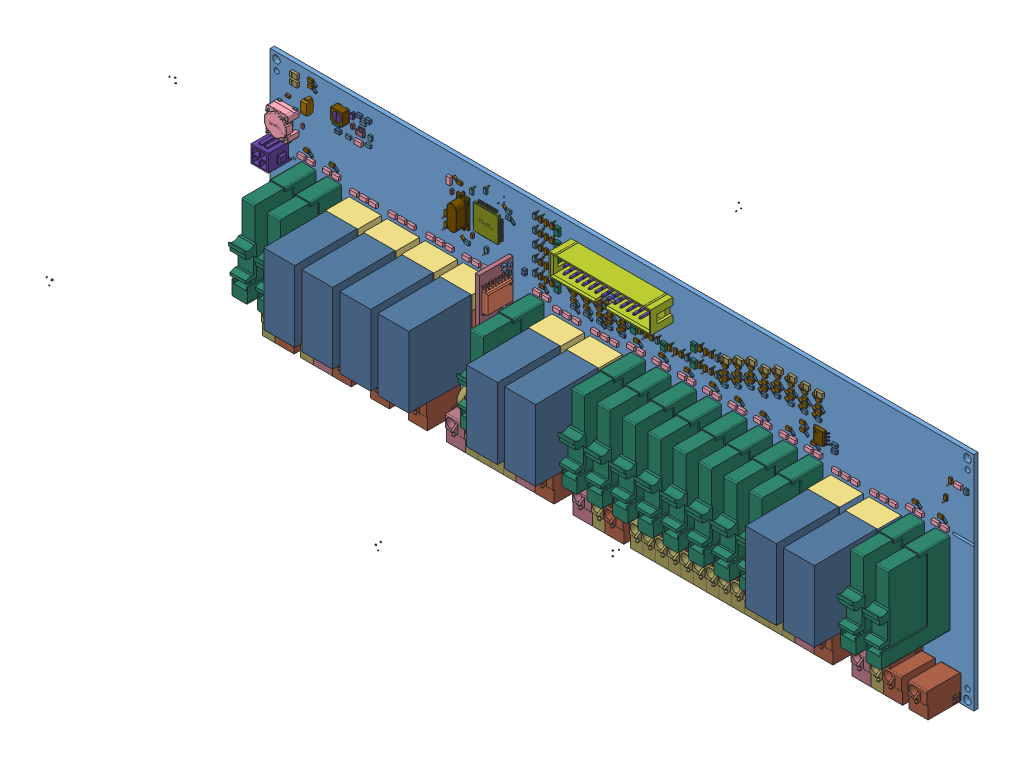
SolidWorks assembly _SC941C, configuration Default. Lengths in mm. (continued)
Components (placement in the parent): (continued)
- R40-1: R40 [Default] at origin size (1.97 3.3 0.78)
  - SW3dPS-0805_SMD_Resistor-1: SW3dPS-0805_SMD_Resistor [Default] at (147.4471 56.8959 0) x (0 -1 0) z (-1 0 0) size (2 0.78 1.25)
  - 905262864-1: 905262864 [Default] at (148.1217 58.6819 0) size (1.35 1.03 0.76)
    - Extruded_11-1: Extruded_11 [Default] at origin size (1.35 1.03 0.76)
  - 905261368-1: 905261368 [Default] at (148.0423 58.4438 0) size (1.51 1.51 0.76)
    - Extruded_12-1: Extruded_12 [Default] at origin size (1.51 1.51 0.76)
  - 905260688-1: 905260688 [Default] at (148.082 58.5629 0) size (1.43 1.11 0.76)
    - Extruded_13-1: Extruded_13 [Default] at origin size (1.43 1.11 0.76)
- R35-1: R35 [Default] at origin size (3.3 1.97 0.78)
  - SW3dPS-0805_SMD_Resistor-1: SW3dPS-0805_SMD_Resistor [Default] at (130.8101 54.2291 0) x (1 0 0) z (0 -1 0) size (2 0.78 1.25)
  - 905266264-1: 905266264 [Default] at (129.0241 54.9037 0) size (1.03 1.35 0.76)
    - Extruded_14-1: Extruded_14 [Default] at origin size (1.03 1.35 0.76)
  - 905263816-1: 905263816 [Default] at (129.2622 54.8243 0) size (1.51 1.51 0.76)
    - Extruded_15-1: Extruded_15 [Default] at origin size (1.51 1.51 0.76)
  - 905266536-1: 905266536 [Default] at (129.1431 54.864 0) size (1.11 1.43 0.76)
    - Extruded_16-1: Extruded_16 [Default] at origin size (1.11 1.43 0.76)
- R33-1: R33 [Default] at origin size (3.3 1.97 0.78)
  - SW3dPS-0805_SMD_Resistor-1: SW3dPS-0805_SMD_Resistor [Default] at (136.0171 54.2291 0) x (1 0 0) z (0 -1 0) size (2 0.78 1.25)
  - 905266264-1: 905266264 [Default] at (134.2311 54.9037 0) size (1.03 1.35 0.76)
    - Extruded_14-1: Extruded_14 [Default] at origin size (1.03 1.35 0.76)
  - 905263816-1: 905263816 [Default] at (134.4692 54.8243 0) size (1.51 1.51 0.76)
    - Extruded_15-1: Extruded_15 [Default] at origin size (1.51 1.51 0.76)
  - 905266536-1: 905266536 [Default] at (134.3501 54.864 0) size (1.11 1.43 0.76)
    - Extruded_16-1: Extruded_16 [Default] at origin size (1.11 1.43 0.76)
- R49-1: R49 [Default] at origin size (1.97 3.3 0.78)
  - SW3dPS-0805_SMD_Resistor-1: SW3dPS-0805_SMD_Resistor [Default] at (154.8131 56.8959 0) x (0 -1 0) z (-1 0 0) size (2 0.78 1.25)
  - 905262864-1: 905262864 [Default] at (155.4877 58.6819 0) size (1.35 1.03 0.76)
    - Extruded_11-1: Extruded_11 [Default] at origin size (1.35 1.03 0.76)
  - 905261368-1: 905261368 [Default] at (155.4083 58.4438 0) size (1.51 1.51 0.76)
    - Extruded_12-1: Extruded_12 [Default] at origin size (1.51 1.51 0.76)
  - 905260688-1: 905260688 [Default] at (155.448 58.5629 0) size (1.43 1.11 0.76)
    - Extruded_13-1: Extruded_13 [Default] at origin size (1.43 1.11 0.76)
- R38-1: R38 [Default] at origin size (1.97 3.3 0.78)
  - SW3dPS-0805_SMD_Resistor-1: SW3dPS-0805_SMD_Resistor [Default] at (142.8751 56.8959 0) x (0 -1 0) z (-1 0 0) size (2 0.78 1.25)
  - 905262864-1: 905262864 [Default] at (143.5497 58.6819 0) size (1.35 1.03 0.76)
    - Extruded_11-1: Extruded_11 [Default] at origin size (1.35 1.03 0.76)
  - 905261368-1: 905261368 [Default] at (143.4703 58.4438 0) size (1.51 1.51 0.76)
    - Extruded_12-1: Extruded_12 [Default] at origin size (1.51 1.51 0.76)
  - 905260688-1: 905260688 [Default] at (143.51 58.5629 0) size (1.43 1.11 0.76)
    - Extruded_13-1: Extruded_13 [Default] at origin size (1.43 1.11 0.76)
- R36-1: R36 [Default] at origin size (3.3 1.97 0.78)
  - SW3dPS-0805_SMD_Resistor-1: SW3dPS-0805_SMD_Resistor [Default] at (130.8101 58.8011 0) x (1 0 0) z (0 -1 0) size (2 0.78 1.25)
  - 905266264-1: 905266264 [Default] at (129.0241 59.4757 0) size (1.03 1.35 0.76)
    - Extruded_14-1: Extruded_14 [Default] at origin size (1.03 1.35 0.76)
  - 905263816-1: 905263816 [Default] at (129.2622 59.3963 0) size (1.51 1.51 0.76)
    - Extruded_15-1: Extruded_15 [Default] at origin size (1.51 1.51 0.76)
  - 905266536-1: 905266536 [Default] at (129.1431 59.436 0) size (1.11 1.43 0.76)
    - Extruded_16-1: Extruded_16 [Default] at origin size (1.11 1.43 0.76)
- R32-1: R32 [Default] at origin size (3.3 1.97 0.78)
  - SW3dPS-0805_SMD_Resistor-1: SW3dPS-0805_SMD_Resistor [Default] at (136.0171 58.8011 0) x (1 0 0) z (0 -1 0) size (2 0.78 1.25)
  - 905266264-1: 905266264 [Default] at (134.2311 59.4757 0) size (1.03 1.35 0.76)
    - Extruded_14-1: Extruded_14 [Default] at origin size (1.03 1.35 0.76)
  - 905263816-1: 905263816 [Default] at (134.4692 59.3963 0) size (1.51 1.51 0.76)
    - Extruded_15-1: Extruded_15 [Default] at origin size (1.51 1.51 0.76)
  - 905266536-1: 905266536 [Default] at (134.3501 59.436 0) size (1.11 1.43 0.76)
    - Extruded_16-1: Extruded_16 [Default] at origin size (1.11 1.43 0.76)
- R17_1-1: R17_1 [Default] at origin size (3.3 1.97 0.78)
  - SW3dPS-0805_SMD_Resistor-1: SW3dPS-0805_SMD_Resistor [Default] at (121.4121 56.5151 0) x (1 0 0) z (0 -1 0) size (2 0.78 1.25)
  - 905266264-1: 905266264 [Default] at (119.6261 57.1897 0) size (1.03 1.35 0.76)
    - Extruded_14-1: Extruded_14 [Default] at origin size (1.03 1.35 0.76)
  - 905263816-1: 905263816 [Default] at (119.8642 57.1103 0) size (1.51 1.51 0.76)
    - Extruded_15-1: Extruded_15 [Default] at origin size (1.51 1.51 0.76)
  - 905266536-1: 905266536 [Default] at (119.7451 57.15 0) size (1.11 1.43 0.76)
    - Extruded_16-1: Extruded_16 [Default] at origin size (1.11 1.43 0.76)
- R11_1-1: R11_1 [Default] at origin size (1.97 3.3 0.78)
  - SW3dPS-0805_SMD_Resistor-1: SW3dPS-0805_SMD_Resistor [Default] at (105.2829 60.7061 0) x (0 1 0) z (1 0 0) size (2 0.78 1.25)
  - 905261640-1: 905261640 [Default] at (104.6083 58.9201 0) size (1.35 1.03 0.76)
    - Extruded_8-1: Extruded_8 [Default] at origin size (1.35 1.03 0.76)
  - 905260416-1: 905260416 [Default] at (104.6877 59.1582 0) size (1.51 1.51 0.76)
    - Extruded_9-1: Extruded_9 [Default] at origin size (1.51 1.51 0.76)
  - 905266128-1: 905266128 [Default] at (104.648 59.0391 0) size (1.43 1.11 0.76)
    - Extruded_10-1: Extruded_10 [Default] at origin size (1.43 1.11 0.76)
- R21-1: R21 [Default] at origin size (3.3 1.97 0.78)
  - SW3dPS-0805_SMD_Resistor-1: SW3dPS-0805_SMD_Resistor [Default] at (116.2049 54.2289 0) x (-1 0 0) z (0 1 0) size (2 0.78 1.25)
  - 905261096-1: 905261096 [Default] at (117.9909 53.5543 0) size (1.03 1.35 0.76)
    - Extruded_2-1: Extruded_2 [Default] at origin size (1.03 1.35 0.76)
  - 905275240-1: 905275240 [Default] at (117.7528 53.6337 0) size (1.51 1.51 0.76)
    - Extruded_3-1: Extruded_3 [Default] at origin size (1.51 1.51 0.76)
  - 905265720-1: 905265720 [Default] at (117.8719 53.594 0) size (1.11 1.43 0.76)
    - Extruded_4-1: Extruded_4 [Default] at origin size (1.11 1.43 0.76)
- R16_1-1: R16_1 [Default] at origin size (3.3 1.97 0.78)
  - SW3dPS-0805_SMD_Resistor-1: SW3dPS-0805_SMD_Resistor [Default] at (121.4119 54.2289 0) x (-1 0 0) z (0 1 0) size (2 0.78 1.25)
  - 905261096-1: 905261096 [Default] at (123.1979 53.5543 0) size (1.03 1.35 0.76)
    - Extruded_2-1: Extruded_2 [Default] at origin size (1.03 1.35 0.76)
  - 905275240-1: 905275240 [Default] at (122.9598 53.6337 0) size (1.51 1.51 0.76)
    - Extruded_3-1: Extruded_3 [Default] at origin size (1.51 1.51 0.76)
  - 905265720-1: 905265720 [Default] at (123.0789 53.594 0) size (1.11 1.43 0.76)
    - Extruded_4-1: Extruded_4 [Default] at origin size (1.11 1.43 0.76)
- R10-1: R10 [Default] at origin size (1.97 3.3 0.78)
  - SW3dPS-0805_SMD_Resistor-1: SW3dPS-0805_SMD_Resistor [Default] at (102.9971 60.7059 0) x (0 -1 0) z (-1 0 0) size (2 0.78 1.25)
  - 905262864-1: 905262864 [Default] at (103.6717 62.4919 0) size (1.35 1.03 0.76)
    - Extruded_11-1: Extruded_11 [Default] at origin size (1.35 1.03 0.76)
  - 905261368-1: 905261368 [Default] at (103.5923 62.2538 0) size (1.51 1.51 0.76)
    - Extruded_12-1: Extruded_12 [Default] at origin size (1.51 1.51 0.76)
  - 905260688-1: 905260688 [Default] at (103.632 62.3729 0) size (1.43 1.11 0.76)
    - Extruded_13-1: Extruded_13 [Default] at origin size (1.43 1.11 0.76)
- R26_1-1: R26_1 [Default] at origin size (3.3 1.97 0.78)
  - SW3dPS-0805_SMD_Resistor-1: SW3dPS-0805_SMD_Resistor [Default] at (126.6189 58.8009 0) x (-1 0 0) z (0 1 0) size (2 0.78 1.25)
  - 905261096-1: 905261096 [Default] at (128.4049 58.1263 0) size (1.03 1.35 0.76)
    - Extruded_2-1: Extruded_2 [Default] at origin size (1.03 1.35 0.76)
  - 905275240-1: 905275240 [Default] at (128.1668 58.2057 0) size (1.51 1.51 0.76)
    - Extruded_3-1: Extruded_3 [Default] at origin size (1.51 1.51 0.76)
  - 905265720-1: 905265720 [Default] at (128.2859 58.166 0) size (1.11 1.43 0.76)
    - Extruded_4-1: Extruded_4 [Default] at origin size (1.11 1.43 0.76)
- R47-1: R47 [Default] at origin size (1.97 3.3 0.78)
  - SW3dPS-0805_SMD_Resistor-1: SW3dPS-0805_SMD_Resistor [Default] at (159.3851 56.8959 0) x (0 -1 0) z (-1 0 0) size (2 0.78 1.25)
  - 905262864-1: 905262864 [Default] at (160.0597 58.6819 0) size (1.35 1.03 0.76)
    - Extruded_11-1: Extruded_11 [Default] at origin size (1.35 1.03 0.76)
  - 905261368-1: 905261368 [Default] at (159.9803 58.4438 0) size (1.51 1.51 0.76)
    - Extruded_12-1: Extruded_12 [Default] at origin size (1.51 1.51 0.76)
  - 905260688-1: 905260688 [Default] at (160.02 58.5629 0) size (1.43 1.11 0.76)
    - Extruded_13-1: Extruded_13 [Default] at origin size (1.43 1.11 0.76)
- R28-1: R28 [Default] at origin size (3.3 1.97 0.78)
  - SW3dPS-0805_SMD_Resistor-1: SW3dPS-0805_SMD_Resistor [Default] at (126.6189 54.2289 0) x (-1 0 0) z (0 1 0) size (2 0.78 1.25)
  - 905261096-1: 905261096 [Default] at (128.4049 53.5543 0) size (1.03 1.35 0.76)
    - Extruded_2-1: Extruded_2 [Default] at origin size (1.03 1.35 0.76)
  - 905275240-1: 905275240 [Default] at (128.1668 53.6337 0) size (1.51 1.51 0.76)
    - Extruded_3-1: Extruded_3 [Default] at origin size (1.51 1.51 0.76)
  - 905265720-1: 905265720 [Default] at (128.2859 53.594 0) size (1.11 1.43 0.76)
    - Extruded_4-1: Extruded_4 [Default] at origin size (1.11 1.43 0.76)
- R30-1: R30 [Default] at origin size (1.97 3.3 0.78)
  - SW3dPS-0805_SMD_Resistor-1: SW3dPS-0805_SMD_Resistor [Default] at (102.9971 55.7529 0) x (0 -1 0) z (-1 0 0) size (2 0.78 1.25)
  - 905262864-1: 905262864 [Default] at (103.6717 57.5389 0) size (1.35 1.03 0.76)
    - Extruded_11-1: Extruded_11 [Default] at origin size (1.35 1.03 0.76)
  - 905261368-1: 905261368 [Default] at (103.5923 57.3008 0) size (1.51 1.51 0.76)
    - Extruded_12-1: Extruded_12 [Default] at origin size (1.51 1.51 0.76)
  - 905260688-1: 905260688 [Default] at (103.632 57.4199 0) size (1.43 1.11 0.76)
    - Extruded_13-1: Extruded_13 [Default] at origin size (1.43 1.11 0.76)
- R23-1: R23 [Default] at origin size (1.97 3.3 0.78)
  - SW3dPS-0805_SMD_Resistor-1: SW3dPS-0805_SMD_Resistor [Default] at (102.9971 75.5649 0) x (0 -1 0) z (-1 0 0) size (2 0.78 1.25)
  - 905262864-1: 905262864 [Default] at (103.6717 77.3509 0) size (1.35 1.03 0.76)
    - Extruded_11-1: Extruded_11 [Default] at origin size (1.35 1.03 0.76)
  - 905261368-1: 905261368 [Default] at (103.5923 77.1128 0) size (1.51 1.51 0.76)
    - Extruded_12-1: Extruded_12 [Default] at origin size (1.51 1.51 0.76)
  - 905260688-1: 905260688 [Default] at (103.632 77.2319 0) size (1.43 1.11 0.76)
    - Extruded_13-1: Extruded_13 [Default] at origin size (1.43 1.11 0.76)
- R18_1-1: R18_1 [Default] at origin size (1.97 3.3 0.78)
  - SW3dPS-0805_SMD_Resistor-1: SW3dPS-0805_SMD_Resistor [Default] at (102.9971 65.6589 0) x (0 -1 0) z (-1 0 0) size (2 0.78 1.25)
  - 905262864-1: 905262864 [Default] at (103.6717 67.4449 0) size (1.35 1.03 0.76)
    - Extruded_11-1: Extruded_11 [Default] at origin size (1.35 1.03 0.76)
  - 905261368-1: 905261368 [Default] at (103.5923 67.2068 0) size (1.51 1.51 0.76)
    - Extruded_12-1: Extruded_12 [Default] at origin size (1.51 1.51 0.76)
  - 905260688-1: 905260688 [Default] at (103.632 67.3259 0) size (1.43 1.11 0.76)
    - Extruded_13-1: Extruded_13 [Default] at origin size (1.43 1.11 0.76)
- R12_1-1: R12_1 [Default] at origin size (1.97 3.3 0.78)
  - SW3dPS-0805_SMD_Resistor-1: SW3dPS-0805_SMD_Resistor [Default] at (102.9971 70.6119 0) x (0 -1 0) z (-1 0 0) size (2 0.78 1.25)
  - 905262864-1: 905262864 [Default] at (103.6717 72.3979 0) size (1.35 1.03 0.76)
    - Extruded_11-1: Extruded_11 [Default] at origin size (1.35 1.03 0.76)
  - 905261368-1: 905261368 [Default] at (103.5923 72.1598 0) size (1.51 1.51 0.76)
    - Extruded_12-1: Extruded_12 [Default] at origin size (1.51 1.51 0.76)
  - 905260688-1: 905260688 [Default] at (103.632 72.2789 0) size (1.43 1.11 0.76)
    - Extruded_13-1: Extruded_13 [Default] at origin size (1.43 1.11 0.76)
- R27-1: R27 [Default] at origin size (1.97 3.3 0.78)
  - SW3dPS-0805_SMD_Resistor-1: SW3dPS-0805_SMD_Resistor [Default] at (107.5691 55.7529 0) x (0 -1 0) z (-1 0 0) size (2 0.78 1.25)
  - 905262864-1: 905262864 [Default] at (108.2437 57.5389 0) size (1.35 1.03 0.76)
    - Extruded_11-1: Extruded_11 [Default] at origin size (1.35 1.03 0.76)
  - 905261368-1: 905261368 [Default] at (108.1643 57.3008 0) size (1.51 1.51 0.76)
    - Extruded_12-1: Extruded_12 [Default] at origin size (1.51 1.51 0.76)
  - 905260688-1: 905260688 [Default] at (108.204 57.4199 0) size (1.43 1.11 0.76)
    - Extruded_13-1: Extruded_13 [Default] at origin size (1.43 1.11 0.76)
- R25_1-1: R25_1 [Default] at origin size (1.97 3.3 0.78)
  - SW3dPS-0805_SMD_Resistor-1: SW3dPS-0805_SMD_Resistor [Default] at (107.5691 75.5649 0) x (0 -1 0) z (-1 0 0) size (2 0.78 1.25)
  - 905262864-1: 905262864 [Default] at (108.2437 77.3509 0) size (1.35 1.03 0.76)
    - Extruded_11-1: Extruded_11 [Default] at origin size (1.35 1.03 0.76)
  - 905261368-1: 905261368 [Default] at (108.1643 77.1128 0) size (1.51 1.51 0.76)
    - Extruded_12-1: Extruded_12 [Default] at origin size (1.51 1.51 0.76)
  - 905260688-1: 905260688 [Default] at (108.204 77.2319 0) size (1.43 1.11 0.76)
    - Extruded_13-1: Extruded_13 [Default] at origin size (1.43 1.11 0.76)
- R15_1-1: R15_1 [Default] at origin size (1.97 3.3 0.78)
  - SW3dPS-0805_SMD_Resistor-1: SW3dPS-0805_SMD_Resistor [Default] at (107.5691 65.6589 0) x (0 -1 0) z (-1 0 0) size (2 0.78 1.25)
  - 905262864-1: 905262864 [Default] at (108.2437 67.4449 0) size (1.35 1.03 0.76)
    - Extruded_11-1: Extruded_11 [Default] at origin size (1.35 1.03 0.76)
  - 905261368-1: 905261368 [Default] at (108.1643 67.2068 0) size (1.51 1.51 0.76)
    - Extruded_12-1: Extruded_12 [Default] at origin size (1.51 1.51 0.76)
  - 905260688-1: 905260688 [Default] at (108.204 67.3259 0) size (1.43 1.11 0.76)
    - Extruded_13-1: Extruded_13 [Default] at origin size (1.43 1.11 0.76)
- R9_1-1: R9_1 [Default] at origin size (1.97 3.3 0.78)
  - SW3dPS-0805_SMD_Resistor-1: SW3dPS-0805_SMD_Resistor [Default] at (107.5691 70.6119 0) x (0 -1 0) z (-1 0 0) size (2 0.78 1.25)
  - 905262864-1: 905262864 [Default] at (108.2437 72.3979 0) size (1.35 1.03 0.76)
    - Extruded_11-1: Extruded_11 [Default] at origin size (1.35 1.03 0.76)
  - 905261368-1: 905261368 [Default] at (108.1643 72.1598 0) size (1.51 1.51 0.76)
    - Extruded_12-1: Extruded_12 [Default] at origin size (1.51 1.51 0.76)
  - 905260688-1: 905260688 [Default] at (108.204 72.2789 0) size (1.43 1.11 0.76)
    - Extruded_13-1: Extruded_13 [Default] at origin size (1.43 1.11 0.76)
- R14-1: R14 [Default] at origin size (3.3 1.97 0.78)
  - SW3dPS-0805_SMD_Resistor-1: SW3dPS-0805_SMD_Resistor [Default] at (121.4119 58.8009 0) x (-1 0 0) z (0 1 0) size (2 0.78 1.25)
  - 905261096-1: 905261096 [Default] at (123.1979 58.1263 0) size (1.03 1.35 0.76)
    - Extruded_2-1: Extruded_2 [Default] at origin size (1.03 1.35 0.76)
  - 905275240-1: 905275240 [Default] at (122.9598 58.2057 0) size (1.51 1.51 0.76)
    - Extruded_3-1: Extruded_3 [Default] at origin size (1.51 1.51 0.76)
  - 905265720-1: 905265720 [Default] at (123.0789 58.166 0) size (1.11 1.43 0.76)
    - Extruded_4-1: Extruded_4 [Default] at origin size (1.11 1.43 0.76)
- R8_1-1: R8_1 [Default] at origin size (1.97 3.3 0.78)
  - SW3dPS-0805_SMD_Resistor-1: SW3dPS-0805_SMD_Resistor [Default] at (107.5691 60.7059 0) x (0 -1 0) z (-1 0 0) size (2 0.78 1.25)
  - 905262864-1: 905262864 [Default] at (108.2437 62.4919 0) size (1.35 1.03 0.76)
    - Extruded_11-1: Extruded_11 [Default] at origin size (1.35 1.03 0.76)
  - 905261368-1: 905261368 [Default] at (108.1643 62.2538 0) size (1.51 1.51 0.76)
    - Extruded_12-1: Extruded_12 [Default] at origin size (1.51 1.51 0.76)
  - 905260688-1: 905260688 [Default] at (108.204 62.3729 0) size (1.43 1.11 0.76)
    - Extruded_13-1: Extruded_13 [Default] at origin size (1.43 1.11 0.76)
- R56-1: R56 [Default] at origin size (3.3 1.97 0.78)
  - SW3dPS-0805_SMD_Resistor-1: SW3dPS-0805_SMD_Resistor [Default] at (171.9262 52.7049 0) x (-1 0 0) z (0 1 0) size (2 0.78 1.25)
  - 905261096-1: 905261096 [Default] at (173.7122 52.0303 0) size (1.03 1.35 0.76)
    - Extruded_2-1: Extruded_2 [Default] at origin size (1.03 1.35 0.76)
  - 905275240-1: 905275240 [Default] at (173.4741 52.1097 0) size (1.51 1.51 0.76)
    - Extruded_3-1: Extruded_3 [Default] at origin size (1.51 1.51 0.76)
  - 905265720-1: 905265720 [Default] at (173.5931 52.07 0) size (1.11 1.43 0.76)
    - Extruded_4-1: Extruded_4 [Default] at origin size (1.11 1.43 0.76)
- R52-1: R52 [Default] at origin size (3.3 1.97 0.78)
  - SW3dPS-0805_SMD_Resistor-1: SW3dPS-0805_SMD_Resistor [Default] at (161.7662 52.7049 0) x (-1 0 0) z (0 1 0) size (2 0.78 1.25)
  - 905261096-1: 905261096 [Default] at (163.5522 52.0303 0) size (1.03 1.35 0.76)
    - Extruded_2-1: Extruded_2 [Default] at origin size (1.03 1.35 0.76)
  - 905275240-1: 905275240 [Default] at (163.3141 52.1097 0) size (1.51 1.51 0.76)
    - Extruded_3-1: Extruded_3 [Default] at origin size (1.51 1.51 0.76)
  - 905265720-1: 905265720 [Default] at (163.4331 52.07 0) size (1.11 1.43 0.76)
    - Extruded_4-1: Extruded_4 [Default] at origin size (1.11 1.43 0.76)
- R71-1: R71 [Default] at origin size (3.3 1.97 0.78)
  - SW3dPS-0805_SMD_Resistor-1: SW3dPS-0805_SMD_Resistor [Default] at (207.9624 55.1311 0) x (-1 0 0) z (0 1 0) size (2 0.78 1.25)
  - 905261096-1: 905261096 [Default] at (209.7484 54.4566 0) size (1.03 1.35 0.76)
    - Extruded_2-1: Extruded_2 [Default] at origin size (1.03 1.35 0.76)
  - 905275240-1: 905275240 [Default] at (209.5103 54.5359 0) size (1.51 1.51 0.76)
    - Extruded_3-1: Extruded_3 [Default] at origin size (1.51 1.51 0.76)
  - 905265720-1: 905265720 [Default] at (209.6294 54.4962 0) size (1.11 1.43 0.76)
    - Extruded_4-1: Extruded_4 [Default] at origin size (1.11 1.43 0.76)
- R70-1: R70 [Default] at origin size (3.3 1.97 0.78)
  - SW3dPS-0805_SMD_Resistor-1: SW3dPS-0805_SMD_Resistor [Default] at (207.9624 57.6712 0) x (-1 0 0) z (0 1 0) size (2 0.78 1.25)
  - 905261096-1: 905261096 [Default] at (209.7484 56.9966 0) size (1.03 1.35 0.76)
    - Extruded_2-1: Extruded_2 [Default] at origin size (1.03 1.35 0.76)
  - 905275240-1: 905275240 [Default] at (209.5103 57.0759 0) size (1.51 1.51 0.76)
    - Extruded_3-1: Extruded_3 [Default] at origin size (1.51 1.51 0.76)
  - 905265720-1: 905265720 [Default] at (209.6294 57.0363 0) size (1.11 1.43 0.76)
    - Extruded_4-1: Extruded_4 [Default] at origin size (1.11 1.43 0.76)
- K13-1: K13 [Default] at origin size (6.2 33 32.7)
  - User_Library-93_11-1: User_Library-93_11 [Default] at (168.985 47.3038 0) x (0 -1 0) z (0 0 1) size (33 6.2 32.7)
- K12-1: K12 [Default] at origin size (6.2 33 32.7)
  - User_Library-93_11-1: User_Library-93_11 [Default] at (158.825 47.3038 0) x (0 -1 0) z (0 0 1) size (33 6.2 32.7)
- K2-1: K2 [Default] at origin size (6.2 33 32.7)
  - User_Library-93_11-1: User_Library-93_11 [Default] at (16.585 47.3038 0) x (0 -1 0) z (0 0 1) size (33 6.2 32.7)
- K15-1: K15 [Default] at origin size (6.2 33 32.7)
  - User_Library-93_11-1: User_Library-93_11 [Default] at (189.305 47.3038 0) x (0 -1 0) z (0 0 1) size (33 6.2 32.7)
- K19-1: K19 [Default] at origin size (13 30.3 34.5)
  - relais_40_61_8_006_0000-1: relais_40_61_8_006_0000 [Default] at (240.665 15.7216 9.5) x (0 1 0) z (1 0 0) size (29 30 12.4)
  - 1151725064-1: 1151725064 [Default] at (240.665 34.225 5) size (13 10 4.5)
    - Extruded_6-1: Extruded_6 [Default] at origin size (13 10 4.5)
  - 1151724928-1: 1151724928 [Default] at (240.665 41.975 0) size (13 5.5 9.5)
    - Extruded_7-1: Extruded_7 [Default] at origin size (13 5.5 9.5)
  - 1151724792-1: 1151724792 [Default] at (240.665 21.825 0) size (13 14.8 9.5)
    - Extruded_5-1: Extruded_5 [Default] at origin size (13 14.8 9.5)
- K18-1: K18 [Default] at origin size (13 30.3 34.5)
  - relais_40_61_8_006_0000-1: relais_40_61_8_006_0000 [Default] at (225.425 15.7216 9.5) x (0 1 0) z (1 0 0) size (29 30 12.4)
  - 1151724792-1: 1151724792 [Default] at (225.425 21.825 0) size (13 14.8 9.5)
    - Extruded_5-1: Extruded_5 [Default] at origin size (13 14.8 9.5)
  - 1151724928-1: 1151724928 [Default] at (225.425 41.975 0) size (13 5.5 9.5)
    - Extruded_7-1: Extruded_7 [Default] at origin size (13 5.5 9.5)
  - 1151725064-1: 1151725064 [Default] at (225.425 34.225 5) size (13 10 4.5)
    - Extruded_6-1: Extruded_6 [Default] at origin size (13 10 4.5)
- K9-1: K9 [Default] at origin size (13 30.3 34.5)
  - relais_40_61_8_006_0000-1: relais_40_61_8_006_0000 [Default] at (128.905 15.7216 9.5) x (0 1 0) z (1 0 0) size (29 30 12.4)
  - 1151725064-1: 1151725064 [Default] at (128.905 34.225 5) size (13 10 4.5)
    - Extruded_6-1: Extruded_6 [Default] at origin size (13 10 4.5)
  - 1151724928-1: 1151724928 [Default] at (128.905 41.975 0) size (13 5.5 9.5)
    - Extruded_7-1: Extruded_7 [Default] at origin size (13 5.5 9.5)
  - 1151724792-1: 1151724792 [Default] at (128.905 21.825 0) size (13 14.8 9.5)
    - Extruded_5-1: Extruded_5 [Default] at origin size (13 14.8 9.5)
- K8-1: K8 [Default] at origin size (13 30.3 34.5)
  - relais_40_61_8_006_0000-1: relais_40_61_8_006_0000 [Default] at (113.665 15.7216 9.5) x (0 1 0) z (1 0 0) size (29 30 12.4)
  - 1151724792-1: 1151724792 [Default] at (113.665 21.825 0) size (13 14.8 9.5)
    - Extruded_5-1: Extruded_5 [Default] at origin size (13 14.8 9.5)
  - 1151724928-1: 1151724928 [Default] at (113.665 41.975 0) size (13 5.5 9.5)
    - Extruded_7-1: Extruded_7 [Default] at origin size (13 5.5 9.5)
  - 1151725064-1: 1151725064 [Default] at (113.665 34.225 5) size (13 10 4.5)
    - Extruded_6-1: Extruded_6 [Default] at origin size (13 10 4.5)
- K6-1: K6 [Default] at origin size (13 30.3 34.5)
  - relais_40_61_8_006_0000-1: relais_40_61_8_006_0000 [Default] at (78.105 15.7216 9.5) x (0 1 0) z (1 0 0) size (29 30 12.4)
  - 1151725064-1: 1151725064 [Default] at (78.105 34.225 5) size (13 10 4.5)
    - Extruded_6-1: Extruded_6 [Default] at origin size (13 10 4.5)
  - 1151724928-1: 1151724928 [Default] at (78.105 41.975 0) size (13 5.5 9.5)
    - Extruded_7-1: Extruded_7 [Default] at origin size (13 5.5 9.5)
  - 1151724792-1: 1151724792 [Default] at (78.105 21.825 0) size (13 14.8 9.5)
    - Extruded_5-1: Extruded_5 [Default] at origin size (13 14.8 9.5)
- K5-1: K5 [Default] at origin size (13 30.3 34.5)
  - relais_40_61_8_006_0000-1: relais_40_61_8_006_0000 [Default] at (62.865 15.7216 9.5) x (0 1 0) z (1 0 0) size (29 30 12.4)
  - 1151724792-1: 1151724792 [Default] at (62.865 21.825 0) size (13 14.8 9.5)
    - Extruded_5-1: Extruded_5 [Default] at origin size (13 14.8 9.5)
  - 1151724928-1: 1151724928 [Default] at (62.865 41.975 0) size (13 5.5 9.5)
    - Extruded_7-1: Extruded_7 [Default] at origin size (13 5.5 9.5)
  - 1151725064-1: 1151725064 [Default] at (62.865 34.225 5) size (13 10 4.5)
    - Extruded_6-1: Extruded_6 [Default] at origin size (13 10 4.5)
- K4-1: K4 [Default] at origin size (13 30.3 34.5)
  - relais_40_61_8_006_0000-1: relais_40_61_8_006_0000 [Default] at (47.625 15.7216 9.5) x (0 1 0) z (1 0 0) size (29 30 12.4)
  - 1151725064-1: 1151725064 [Default] at (47.625 34.225 5) size (13 10 4.5)
    - Extruded_6-1: Extruded_6 [Default] at origin size (13 10 4.5)
  - 1151724928-1: 1151724928 [Default] at (47.625 41.975 0) size (13 5.5 9.5)
    - Extruded_7-1: Extruded_7 [Default] at origin size (13 5.5 9.5)
  - 1151724792-1: 1151724792 [Default] at (47.625 21.825 0) size (13 14.8 9.5)
    - Extruded_5-1: Extruded_5 [Default] at origin size (13 14.8 9.5)
- K3-1: K3 [Default] at origin size (13 30.3 34.5)
  - relais_40_61_8_006_0000-1: relais_40_61_8_006_0000 [Default] at (32.385 15.7216 9.5) x (0 1 0) z (1 0 0) size (29 30 12.4)
  - 1151724792-1: 1151724792 [Default] at (32.385 21.825 0) size (13 14.8 9.5)
    - Extruded_5-1: Extruded_5 [Default] at origin size (13 14.8 9.5)
  - 1151724928-1: 1151724928 [Default] at (32.385 41.975 0) size (13 5.5 9.5)
    - Extruded_7-1: Extruded_7 [Default] at origin size (13 5.5 9.5)
  - 1151725064-1: 1151725064 [Default] at (32.385 34.225 5) size (13 10 4.5)
    - Extruded_6-1: Extruded_6 [Default] at origin size (13 10 4.5)
- J96-1: J96 [Default] at origin size (7.62 10 19.2)
  - 1790487-1: 1790487 [Default] at (256.945 -15.67 -10.6) x (0 1 0) z (1 0 0) size (10 19.2 7.62)
    - ffkdsa1-v2-7.62-1: ffkdsa1-v2-7.62 [Default] at (-15.6914 -27.508 9.12) x (0 -1 0) z (0 0 1) size (19.2 10 7.62)
- J93-1: J93 [Default] at origin size (7.62 10 19.2)
  - 1790487-1: 1790487 [Default] at (246.785 -15.67 -10.6) x (0 1 0) z (1 0 0) size (10 19.2 7.62)
    - ffkdsa1-v2-7.62-1: ffkdsa1-v2-7.62 [Default] at (-15.6914 -27.508 9.12) x (0 -1 0) z (0 0 1) size (19.2 10 7.62)
- J91-1: J91 [Default] at origin size (6.88 10 19.2)
  - 1790348-1: 1790348 [Default] at (253.3651 -7.6199 0) x (0 1 0) z (1 0 0) size (10 19.2 6.88)
    - ffkds-v2-5.08-1: ffkds-v2-5.08 [Default] at (-23.7414 -38.158 -2.54) x (0 -1 0) z (0 0 1) size (19.2 10 6.88)
- J88-1: J88 [Default] at origin size (9.42 10 19.2)
  - 1790377-1: 1790377 [Default] at (248.2851 -7.6199 0) x (0 1 0) z (1 0 0) size (10 19.2 9.42)
    - ffkdsa-v2-7.62-1: ffkdsa-v2-7.62 [Default] at (-23.7414 -38.158 -5.08) x (0 -1 0) z (0 0 1) size (19.2 10 9.42)
- J85-1: J85 [Default] at origin size (7.62 10 19.2)
  - 1790487-1: 1790487 [Default] at (218.845 -15.67 -10.6) x (0 1 0) z (1 0 0) size (10 19.2 7.62)
    - ffkdsa1-v2-7.62-1: ffkdsa1-v2-7.62 [Default] at (-15.6914 -27.508 9.12) x (0 -1 0) z (0 0 1) size (19.2 10 7.62)
- J83-1: J83 [Default] at origin size (9.42 10 19.2)
  - 1790377-1: 1790377 [Default] at (225.425 -7.6199 0) x (0 1 0) z (1 0 0) size (10 19.2 9.42)
    - ffkdsa-v2-7.62-1: ffkdsa-v2-7.62 [Default] at (-23.7414 -38.158 -5.08) x (0 -1 0) z (0 0 1) size (19.2 10 9.42)
- J80-1: J80 [Default] at origin size (6.88 10 19.2)
  - 1790348-1: 1790348 [Default] at (217.8051 -7.6199 0) x (0 1 0) z (1 0 0) size (10 19.2 6.88)
    - ffkds-v2-5.08-1: ffkds-v2-5.08 [Default] at (-23.7414 -38.158 -2.54) x (0 -1 0) z (0 0 1) size (19.2 10 6.88)
- J78-1: J78 [Default] at origin size (6.88 10 19.2)
  - 1790348-1: 1790348 [Default] at (212.7251 -7.6199 0) x (0 1 0) z (1 0 0) size (10 19.2 6.88)
    - ffkds-v2-5.08-1: ffkds-v2-5.08 [Default] at (-23.7414 -38.158 -2.54) x (0 -1 0) z (0 0 1) size (19.2 10 6.88)
- J75-1: J75 [Default] at origin size (6.88 10 19.2)
  - 1790348-1: 1790348 [Default] at (207.6451 -7.6199 0) x (0 1 0) z (1 0 0) size (10 19.2 6.88)
    - ffkds-v2-5.08-1: ffkds-v2-5.08 [Default] at (-23.7414 -38.158 -2.54) x (0 -1 0) z (0 0 1) size (19.2 10 6.88)
- J73-1: J73 [Default] at origin size (6.88 10 19.2)
  - 1790348-1: 1790348 [Default] at (202.5651 -7.6199 0) x (0 1 0) z (1 0 0) size (10 19.2 6.88)
    - ffkds-v2-5.08-1: ffkds-v2-5.08 [Default] at (-23.7414 -38.158 -2.54) x (0 -1 0) z (0 0 1) size (19.2 10 6.88)
- J70-1: J70 [Default] at origin size (6.88 10 19.2)
  - 1790348-1: 1790348 [Default] at (197.4851 -7.6199 0) x (0 1 0) z (1 0 0) size (10 19.2 6.88)
    - ffkds-v2-5.08-1: ffkds-v2-5.08 [Default] at (-23.7414 -38.158 -2.54) x (0 -1 0) z (0 0 1) size (19.2 10 6.88)
- J68-1: J68 [Default] at origin size (6.88 10 19.2)
  - 1790348-1: 1790348 [Default] at (192.4051 -7.6199 0) x (0 1 0) z (1 0 0) size (10 19.2 6.88)
    - ffkds-v2-5.08-1: ffkds-v2-5.08 [Default] at (-23.7414 -38.158 -2.54) x (0 -1 0) z (0 0 1) size (19.2 10 6.88)
- J65-1: J65 [Default] at origin size (6.88 10 19.2)
  - 1790348-1: 1790348 [Default] at (187.3251 -7.6199 0) x (0 1 0) z (1 0 0) size (10 19.2 6.88)
    - ffkds-v2-5.08-1: ffkds-v2-5.08 [Default] at (-23.7414 -38.158 -2.54) x (0 -1 0) z (0 0 1) size (19.2 10 6.88)
- J63-1: J63 [Default] at origin size (6.88 10 19.2)
  - 1790348-1: 1790348 [Default] at (182.2451 -7.6199 0) x (0 1 0) z (1 0 0) size (10 19.2 6.88)
    - ffkds-v2-5.08-1: ffkds-v2-5.08 [Default] at (-23.7414 -38.158 -2.54) x (0 -1 0) z (0 0 1) size (19.2 10 6.88)
- J60-1: J60 [Default] at origin size (6.88 10 19.2)
  - 1790348-1: 1790348 [Default] at (177.1651 -7.6199 0) x (0 1 0) z (1 0 0) size (10 19.2 6.88)
    - ffkds-v2-5.08-1: ffkds-v2-5.08 [Default] at (-23.7414 -38.158 -2.54) x (0 -1 0) z (0 0 1) size (19.2 10 6.88)
- J58-1: J58 [Default] at origin size (6.88 10 19.2)
  - 1790348-1: 1790348 [Default] at (172.0851 -7.6199 0) x (0 1 0) z (1 0 0) size (10 19.2 6.88)
    - ffkds-v2-5.08-1: ffkds-v2-5.08 [Default] at (-23.7414 -38.158 -2.54) x (0 -1 0) z (0 0 1) size (19.2 10 6.88)
- J55-1: J55 [Default] at origin size (6.88 10 19.2)
  - 1790348-1: 1790348 [Default] at (167.0051 -7.6199 0) x (0 1 0) z (1 0 0) size (10 19.2 6.88)
    - ffkds-v2-5.08-1: ffkds-v2-5.08 [Default] at (-23.7414 -38.158 -2.54) x (0 -1 0) z (0 0 1) size (19.2 10 6.88)
- J53-1: J53 [Default] at origin size (6.88 10 19.2)
  - 1790348-1: 1790348 [Default] at (161.9251 -7.6199 0) x (0 1 0) z (1 0 0) size (10 19.2 6.88)
    - ffkds-v2-5.08-1: ffkds-v2-5.08 [Default] at (-23.7414 -38.158 -2.54) x (0 -1 0) z (0 0 1) size (19.2 10 6.88)
- J50-1: J50 [Default] at origin size (6.88 10 19.2)
  - 1790348-1: 1790348 [Default] at (156.8451 -7.6199 0) x (0 1 0) z (1 0 0) size (10 19.2 6.88)
    - ffkds-v2-5.08-1: ffkds-v2-5.08 [Default] at (-23.7414 -38.158 -2.54) x (0 -1 0) z (0 0 1) size (19.2 10 6.88)
- J47-1: J47 [Default] at origin size (7.62 10 19.2)
  - 1790487-1: 1790487 [Default] at (135.025 -15.67 -10.6) x (0 1 0) z (1 0 0) size (10 19.2 7.62)
    - ffkdsa1-v2-7.62-1: ffkdsa1-v2-7.62 [Default] at (-15.6914 -27.508 9.12) x (0 -1 0) z (0 0 1) size (19.2 10 7.62)
- J45-1: J45 [Default] at origin size (6.88 10 19.2)
  - 1790348-1: 1790348 [Default] at (141.6051 -7.6199 0) x (0 1 0) z (1 0 0) size (10 19.2 6.88)
    - ffkds-v2-5.08-1: ffkds-v2-5.08 [Default] at (-23.7414 -38.158 -2.54) x (0 -1 0) z (0 0 1) size (19.2 10 6.88)
- J42-1: J42 [Default] at origin size (9.42 10 19.2)
  - 1790377-1: 1790377 [Default] at (136.5251 -7.6199 0) x (0 1 0) z (1 0 0) size (10 19.2 9.42)
    - ffkdsa-v2-7.62-1: ffkdsa-v2-7.62 [Default] at (-23.7414 -38.158 -5.08) x (0 -1 0) z (0 0 1) size (19.2 10 9.42)
- J39-1: J39 [Default] at origin size (7.62 10 19.2)
  - 1790487-1: 1790487 [Default] at (107.085 -15.67 -10.6) x (0 1 0) z (1 0 0) size (10 19.2 7.62)
    - ffkdsa1-v2-7.62-1: ffkdsa1-v2-7.62 [Default] at (-15.6914 -27.508 9.12) x (0 -1 0) z (0 0 1) size (19.2 10 7.62)
- J37-1: J37 [Default] at origin size (9.42 10 19.2)
  - 1790377-1: 1790377 [Default] at (113.6651 -7.6199 0) x (0 1 0) z (1 0 0) size (10 19.2 9.42)
    - ffkdsa-v2-7.62-1: ffkdsa-v2-7.62 [Default] at (-23.7414 -38.158 -5.08) x (0 -1 0) z (0 0 1) size (19.2 10 9.42)
- J34-1: J34 [Default] at origin size (6.88 10 19.2)
  - 1790348-1: 1790348 [Default] at (106.0451 -7.6199 0) x (0 1 0) z (1 0 0) size (10 19.2 6.88)
    - ffkds-v2-5.08-1: ffkds-v2-5.08 [Default] at (-23.7414 -38.158 -2.54) x (0 -1 0) z (0 0 1) size (19.2 10 6.88)
- J31-1: J31 [Default] at origin size (7.62 10 19.2)
  - 1790487-1: 1790487 [Default] at (89.305 -5.67 -10.6) x (0 1 0) z (1 0 0) size (10 19.2 7.62)
    - ffkdsa1-v2-7.62-1: ffkdsa1-v2-7.62 [Default] at (-15.6914 -27.508 9.12) x (0 -1 0) z (0 0 1) size (19.2 10 7.62)
- J27-1: J27 [Default] at origin size (6.88 10 19.2)
  - 1790348-1: 1790348 [Default] at (90.8051 -7.6199 0) x (0 1 0) z (1 0 0) size (10 19.2 6.88)
    - ffkds-v2-5.08-1: ffkds-v2-5.08 [Default] at (-23.7414 -38.158 -2.54) x (0 -1 0) z (0 0 1) size (19.2 10 6.88)
- J24-1: J24 [Default] at origin size (9.42 10 19.2)
  - 1790377-1: 1790377 [Default] at (85.7251 -7.6199 0) x (0 1 0) z (1 0 0) size (10 19.2 9.42)
    - ffkdsa-v2-7.62-1: ffkdsa-v2-7.62 [Default] at (-23.7414 -38.158 -5.08) x (0 -1 0) z (0 0 1) size (19.2 10 9.42)
- J21-1: J21 [Default] at origin size (7.62 10 19.2)
  - 1790487-1: 1790487 [Default] at (56.285 -15.67 -10.6) x (0 1 0) z (1 0 0) size (10 19.2 7.62)
    - ffkdsa1-v2-7.62-1: ffkdsa1-v2-7.62 [Default] at (-15.6914 -27.508 9.12) x (0 -1 0) z (0 0 1) size (19.2 10 7.62)
- J18-1: J18 [Default] at origin size (7.62 10 19.2)
  - 1790487-1: 1790487 [Default] at (41.045 -15.67 -10.6) x (0 1 0) z (1 0 0) size (10 19.2 7.62)
    - ffkdsa1-v2-7.62-1: ffkdsa1-v2-7.62 [Default] at (-15.6914 -27.508 9.12) x (0 -1 0) z (0 0 1) size (19.2 10 7.62)
- J15-1: J15 [Default] at origin size (7.62 10 19.2)
  - 1790487-1: 1790487 [Default] at (25.805 -15.67 -10.6) x (0 1 0) z (1 0 0) size (10 19.2 7.62)
    - ffkdsa1-v2-7.62-1: ffkdsa1-v2-7.62 [Default] at (-15.6914 -27.508 9.12) x (0 -1 0) z (0 0 1) size (19.2 10 7.62)
- J13-1: J13 [Default] at origin size (9.42 10 19.2)
  - 1790377-1: 1790377 [Default] at (32.3851 -7.6199 0) x (0 1 0) z (1 0 0) size (10 19.2 9.42)
    - ffkdsa-v2-7.62-1: ffkdsa-v2-7.62 [Default] at (-23.7414 -38.158 -5.08) x (0 -1 0) z (0 0 1) size (19.2 10 9.42)
- J10-1: J10 [Default] at origin size (6.88 10 19.2)
  - 1790348-1: 1790348 [Default] at (24.7651 -7.6199 0) x (0 1 0) z (1 0 0) size (10 19.2 6.88)
    - ffkds-v2-5.08-1: ffkds-v2-5.08 [Default] at (-23.7414 -38.158 -2.54) x (0 -1 0) z (0 0 1) size (19.2 10 6.88)
- J7-1: J7 [Default] at origin size (7.62 10 19.2)
  - 1790487-1: 1790487 [Default] at (2.945 -15.67 -10.6) x (0 1 0) z (1 0 0) size (10 19.2 7.62)
    - ffkdsa1-v2-7.62-1: ffkdsa1-v2-7.62 [Default] at (-15.6914 -27.508 9.12) x (0 -1 0) z (0 0 1) size (19.2 10 7.62)
- J5-1: J5 [Default] at origin size (6.88 10 19.2)
  - 1790348-1: 1790348 [Default] at (9.5251 -7.6199 0) x (0 1 0) z (1 0 0) size (10 19.2 6.88)
    - ffkds-v2-5.08-1: ffkds-v2-5.08 [Default] at (-23.7414 -38.158 -2.54) x (0 -1 0) z (0 0 1) size (19.2 10 6.88)
- J90-1: J90 [Default] at origin size (7.62 10 19.2)
  - 1790487-1: 1790487 [Default] at (241.705 -5.67 -10.6) x (0 1 0) z (1 0 0) size (10 19.2 7.62)
    - ffkdsa1-v2-7.62-1: ffkdsa1-v2-7.62 [Default] at (-15.6914 -27.508 9.12) x (0 -1 0) z (0 0 1) size (19.2 10 7.62)
- J82-1: J82 [Default] at origin size (7.62 10 19.2)
  - 1790487-1: 1790487 [Default] at (211.225 -5.67 -10.6) x (0 1 0) z (1 0 0) size (10 19.2 7.62)
    - ffkdsa1-v2-7.62-1: ffkdsa1-v2-7.62 [Default] at (-15.6914 -27.508 9.12) x (0 -1 0) z (0 0 1) size (19.2 10 7.62)
- J77-1: J77 [Default] at origin size (7.62 10 19.2)
  - 1790487-1: 1790487 [Default] at (201.065 -5.67 -10.6) x (0 1 0) z (1 0 0) size (10 19.2 7.62)
    - ffkdsa1-v2-7.62-1: ffkdsa1-v2-7.62 [Default] at (-15.6914 -27.508 9.12) x (0 -1 0) z (0 0 1) size (19.2 10 7.62)
- J72-1: J72 [Default] at origin size (7.62 10 19.2)
  - 1790487-1: 1790487 [Default] at (190.905 -5.67 -10.6) x (0 1 0) z (1 0 0) size (10 19.2 7.62)
    - ffkdsa1-v2-7.62-1: ffkdsa1-v2-7.62 [Default] at (-15.6914 -27.508 9.12) x (0 -1 0) z (0 0 1) size (19.2 10 7.62)
- J67-1: J67 [Default] at origin size (7.62 10 19.2)
  - 1790487-1: 1790487 [Default] at (180.745 -5.67 -10.6) x (0 1 0) z (1 0 0) size (10 19.2 7.62)
    - ffkdsa1-v2-7.62-1: ffkdsa1-v2-7.62 [Default] at (-15.6914 -27.508 9.12) x (0 -1 0) z (0 0 1) size (19.2 10 7.62)
- J62-1: J62 [Default] at origin size (7.62 10 19.2)
  - 1790487-1: 1790487 [Default] at (170.585 -5.67 -10.6) x (0 1 0) z (1 0 0) size (10 19.2 7.62)
    - ffkdsa1-v2-7.62-1: ffkdsa1-v2-7.62 [Default] at (-15.6914 -27.508 9.12) x (0 -1 0) z (0 0 1) size (19.2 10 7.62)
- J57-1: J57 [Default] at origin size (7.62 10 19.2)
  - 1790487-1: 1790487 [Default] at (160.425 -5.67 -10.6) x (0 1 0) z (1 0 0) size (10 19.2 7.62)
    - ffkdsa1-v2-7.62-1: ffkdsa1-v2-7.62 [Default] at (-15.6914 -27.508 9.12) x (0 -1 0) z (0 0 1) size (19.2 10 7.62)
- J52-1: J52 [Default] at origin size (7.62 10 19.2)
  - 1790487-1: 1790487 [Default] at (150.265 -5.67 -10.6) x (0 1 0) z (1 0 0) size (10 19.2 7.62)
    - ffkdsa1-v2-7.62-1: ffkdsa1-v2-7.62 [Default] at (-15.6914 -27.508 9.12) x (0 -1 0) z (0 0 1) size (19.2 10 7.62)
- J44-1: J44 [Default] at origin size (7.62 10 19.2)
  - 1790487-1: 1790487 [Default] at (129.945 -5.67 -10.6) x (0 1 0) z (1 0 0) size (10 19.2 7.62)
    - ffkdsa1-v2-7.62-1: ffkdsa1-v2-7.62 [Default] at (-15.6914 -27.508 9.12) x (0 -1 0) z (0 0 1) size (19.2 10 7.62)
- J36-1: J36 [Default] at origin size (7.62 10 19.2)
  - 1790487-1: 1790487 [Default] at (99.465 -5.67 -10.6) x (0 1 0) z (1 0 0) size (10 19.2 7.62)
    - ffkdsa1-v2-7.62-1: ffkdsa1-v2-7.62 [Default] at (-15.6914 -27.508 9.12) x (0 -1 0) z (0 0 1) size (19.2 10 7.62)
- J26-1: J26 [Default] at origin size (7.62 10 19.2)
  - 1790487-1: 1790487 [Default] at (79.145 -5.67 -10.6) x (0 1 0) z (1 0 0) size (10 19.2 7.62)
    - ffkdsa1-v2-7.62-1: ffkdsa1-v2-7.62 [Default] at (-15.6914 -27.508 9.12) x (0 -1 0) z (0 0 1) size (19.2 10 7.62)
- J12-1: J12 [Default] at origin size (7.62 10 19.2)
  - 1790487-1: 1790487 [Default] at (18.185 -5.67 -10.6) x (0 1 0) z (1 0 0) size (10 19.2 7.62)
    - ffkdsa1-v2-7.62-1: ffkdsa1-v2-7.62 [Default] at (-15.6914 -27.508 9.12) x (0 -1 0) z (0 0 1) size (19.2 10 7.62)
- J4-1: J4 [Default] at origin size (7.62 10 19.2)
  - 1790487-1: 1790487 [Default] at (-2.135 -5.67 -10.6) x (0 1 0) z (1 0 0) size (10 19.2 7.62)
    - ffkdsa1-v2-7.62-1: ffkdsa1-v2-7.62 [Default] at (-15.6914 -27.508 9.12) x (0 -1 0) z (0 0 1) size (19.2 10 7.62)
- DL1-1: DL1 [Default] at origin size (1.27 2.03 1.11)
  - SW3dPS-led805-1: SW3dPS-led805 [Default] at (273.6851 66.3799 0) x (1 0 0) z (0 -1 0) size (1.27 1.11 2.03)
- D2_1-1: D2_1 [Default] at origin size (2.9 1.9 0.99)
  - 905269392-1: 905269392 [Default] at (4.4767 73.803 0) size (2.9 1.9 0.98)
    - Extruded_17-1: Extruded_17 [Default] at origin size (2.9 1.9 0.98)
  - 905269800-1: 905269800 [Default] at (3.8418 73.803 0.95) size (0.25 1.78 0.04)
    - Extruded_18-1: Extruded_18 [Default] at origin size (0.25 1.78 0.04)
- D1_1-1: D1_1 [Default] at origin size (2.9 1.9 0.99)
  - 905269392-1: 905269392 [Default] at (4.4767 76.5018 0) size (2.9 1.9 0.98)
    - Extruded_17-1: Extruded_17 [Default] at origin size (2.9 1.9 0.98)
  - 905269800-1: 905269800 [Default] at (3.8418 76.5018 0.95) size (0.25 1.78 0.04)
    - Extruded_18-1: Extruded_18 [Default] at origin size (0.25 1.78 0.04)
- D45-1: D45 [Default] at origin size (2.9 1.9 0.99)
  - 905269392-1: 905269392 [Default] at (187.833 68.707 0) size (2.9 1.9 0.98)
    - Extruded_17-1: Extruded_17 [Default] at origin size (2.9 1.9 0.98)
  - 905269800-1: 905269800 [Default] at (187.198 68.707 0.95) size (0.25 1.78 0.04)
    - Extruded_18-1: Extruded_18 [Default] at origin size (0.25 1.78 0.04)
- D43-1: D43 [Default] at origin size (2.9 1.9 0.99)
  - 905269392-1: 905269392 [Default] at (203.962 70.993 0) size (2.9 1.9 0.98)
    - Extruded_17-1: Extruded_17 [Default] at origin size (2.9 1.9 0.98)
  - 905269800-1: 905269800 [Default] at (203.327 70.993 0.95) size (0.25 1.78 0.04)
    - Extruded_18-1: Extruded_18 [Default] at origin size (0.25 1.78 0.04)
- D41-1: D41 [Default] at origin size (2.9 1.9 0.99)
  - 905269392-1: 905269392 [Default] at (182.626 66.421 0) size (2.9 1.9 0.98)
    - Extruded_17-1: Extruded_17 [Default] at origin size (2.9 1.9 0.98)
  - 905269800-1: 905269800 [Default] at (181.991 66.421 0.95) size (0.25 1.78 0.04)
    - Extruded_18-1: Extruded_18 [Default] at origin size (0.25 1.78 0.04)
- D39-1: D39 [Default] at origin size (2.9 1.9 0.99)
  - 905269392-1: 905269392 [Default] at (209.423 70.993 0) size (2.9 1.9 0.98)
    - Extruded_17-1: Extruded_17 [Default] at origin size (2.9 1.9 0.98)
  - 905269800-1: 905269800 [Default] at (208.788 70.993 0.95) size (0.25 1.78 0.04)
    - Extruded_18-1: Extruded_18 [Default] at origin size (0.25 1.78 0.04)
- D37-1: D37 [Default] at origin size (2.9 1.9 0.99)
  - 905269392-1: 905269392 [Default] at (177.419 64.135 0) size (2.9 1.9 0.98)
    - Extruded_17-1: Extruded_17 [Default] at origin size (2.9 1.9 0.98)
  - 905269800-1: 905269800 [Default] at (176.784 64.135 0.95) size (0.25 1.78 0.04)
    - Extruded_18-1: Extruded_18 [Default] at origin size (0.25 1.78 0.04)
- D35-1: D35 [Default] at origin size (2.9 1.9 0.99)
  - 905269392-1: 905269392 [Default] at (214.884 70.993 0) size (2.9 1.9 0.98)
    - Extruded_17-1: Extruded_17 [Default] at origin size (2.9 1.9 0.98)
  - 905269800-1: 905269800 [Default] at (214.249 70.993 0.95) size (0.25 1.78 0.04)
    - Extruded_18-1: Extruded_18 [Default] at origin size (0.25 1.78 0.04)
